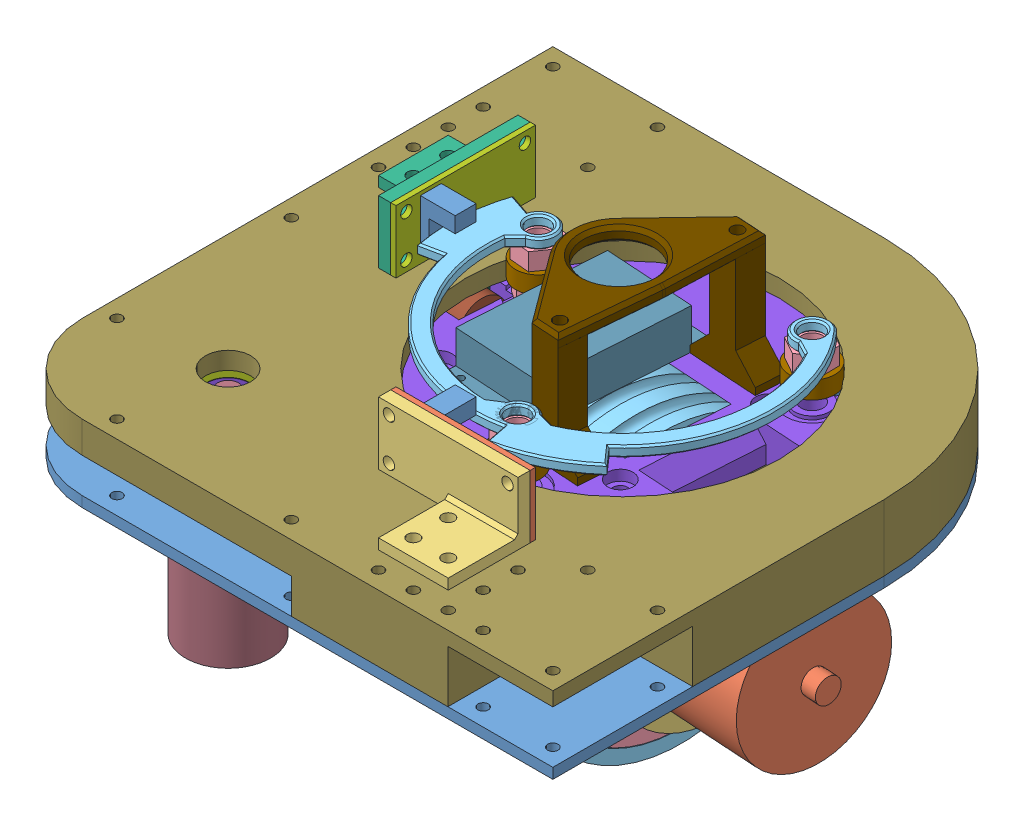
SolidWorks assembly st, configuration ﾃﾞﾌｫﾙﾄ. Lengths in mm.
Overall size (160 121.43 160).
34 component instances, 25 part files, 91 mates.
Components (placement in the parent):
- Copy of st2_base_l^st-1: Copy of st2_base_l^st [ﾃﾞﾌｫﾙﾄ] at (-18.8762 42.7582 -10) x (1 0 0) z (0 1 0) size (160 160 3) (virtual)
- Copy of Copy of 足回りモータ^st-1: Copy of Copy of 足回りモータ^st [ﾃﾞﾌｫﾙﾄ] at (-26.8603 18.2582 -10.5046) x (0 1 0) z (0.063076 0 -0.998009) size (42 98.4 42) (virtual)
- Part5^st-1: Part5^st [ﾃﾞﾌｫﾙﾄ] at (-26.8603 18.2582 -10.5046) x (0 -1 0) z (-0.998009 0 -0.063076) size (57 54 38) (virtual)
- Copy of Part1^st-1: Copy of Part1^st [ﾃﾞﾌｫﾙﾄ] at (-1.01 -10.8145 -54.8758) x (0.057768 -0.401507 -0.914032) z (-0.998009 0 -0.063076) size (72 72 12) (virtual)
- Part7^st-1: Part7^st [ﾃﾞﾌｫﾙﾄ] at (-26.6079 18.2582 -14.4966) x (0 1 0) z (0.063076 0 -0.998009) size (80 42 80) (virtual)
- Part8^st-1: Part8^st [ﾃﾞﾌｫﾙﾄ] at (-54.8045 18.2582 -12.2707) x (0.046572 -0.674423 -0.736875) z (-0.998009 0 -0.063076) size (26 26 8) (virtual)
- Part9^st-1: Part9^st [ﾃﾞﾌｫﾙﾄ] at (-54.8045 18.2582 -12.2707) x (0 -1 0) z (-0.998009 0 -0.063076) size (48 50 11) (virtual)
- Part10^st-1: Part10^st [ﾃﾞﾌｫﾙﾄ] at (-26.8603 48.2582 -10.5046) x (-0.998009 0 -0.063076) z (0 1 0) size (98.93 99.5 10) (virtual)
- Copy of Assem4^st-1: Copy of Assem4^st [ﾃﾞﾌｫﾙﾄ] at (210.0035 137.7188 42.496) x (0.981351 0 0.192225) z (-0.192225 0 0.981351) (virtual)
- Copy of Copy of Copy of Copy (3) of Part3^st-1: Copy of Copy of Copy of Copy (3) of Part3^st [ﾃﾞﾌｫﾙﾄ] at (0.121 53.2582 28.2971) x (0.124113 0.990356 -0.061566) z (0.444379 0 0.895839) size (13 13 5) (virtual)
- Copy (2) of Copy of Copy of Copy (3) of Part3^st-2: Copy (2) of Copy of Copy of Copy (3) of Part3^st [ﾃﾞﾌｫﾙﾄ] at (4.7915 53.2582 -45.6006) x (0.32156 0.922442 0.213776) z (0.55363 0 -0.832763) size (13 13 5) (virtual)
- Copy (3) of Copy of Copy of Copy (3) of Part3^st-3: Copy (3) of Copy of Copy of Copy (3) of Part3^st [ﾃﾞﾌｫﾙﾄ] at (-66.5311 53.2582 -13.0119) x (-0.024356 0.922442 0.385367) z (0.998009 0 0.063076) size (13 13 5) (virtual)
- Copy of st2_base_u^st-1: Copy of st2_base_u^st [ﾃﾞﾌｫﾙﾄ] at (-18.8762 59.7582 -10) x (1 0 0) z (0 1 0) size (160 160 19) (virtual)
- Copy of Copy of Copy of Copy (3) of Part3^st-2: Copy of Copy of Copy of Copy (3) of Part3^st [ﾃﾞﾌｫﾙﾄ] at (-55.3618 63.2582 -22.2904) x (-0.478032 0 0.878342) z (0 1 0) size (13 13 5) (virtual)
- Copy of Copy of Copy of Copy (3) of Part3^st-3: Copy of Copy of Copy of Copy (3) of Part3^st [ﾃﾞﾌｫﾙﾄ] at (10.0104 63.2582 -35.4522) x (0.874344 0 0.485306) z (0 1 0) size (13 13 5) (virtual)
- Copy of Copy of Copy of Copy (3) of Part3^st-4: Copy of Copy of Copy of Copy (3) of Part3^st [ﾃﾞﾌｫﾙﾄ] at (-11.2772 63.2582 27.7426) x (0.840503 0 0.541806) z (0 1 0) size (13 13 5) (virtual)
- Part30^st-1: Part30^st [ﾃﾞﾌｫﾙﾄ] at (-106.4764 42.7582 -41.574) x (-0.707107 0 0.707107) z (0 -1 0) size (24.4 24.4 60.8) (virtual)
- Part31^st-1: Part31^st [ﾃﾞﾌｫﾙﾄ] at (30.1273 58.2582 33.0552) x (-0.998009 0 -0.063076) z (0 1 0) size (25.8 49.4 11.5) (virtual)
- Copy of st2_stgr^st-1: Copy of st2_stgr^st [ﾃﾞﾌｫﾙﾄ] at (-37.084 1 -21.1707) x (-0.998009 0 -0.063076) z (0.063076 0 -0.998009) size (121.99 10 121.99) (virtual)
- Copy of st2_stgr2^st-1: Copy of st2_stgr2^st [ﾃﾞﾌｫﾙﾄ] at (-144.7938 -39.0873 81.6755) x (-1 0 0) z (0 0 -1) size (42 10 42) (virtual)
- Copy of Part10^st-1: Copy of Part10^st [ﾃﾞﾌｫﾙﾄ] at (-73.8405 58.2582 86.1807) x (1 0 0) z (0 -1 0) size (12 12 5) (virtual)
- Part32^st-1: Part32^st [ﾃﾞﾌｫﾙﾄ] at (-28.1078 58.2582 -10.5835) x (-0.998009 0 -0.063076) z (0 1 0) size (33.25 56 34) (virtual)
- Part33^st-1: Part33^st [ﾃﾞﾌｫﾙﾄ] at (-11.7253 224.5363 45) x (-1 0 0) z (0 0 -1) size (6 14 10) (virtual)
- Part34^st-1: Part34^st [ﾃﾞﾌｫﾙﾄ] at (12.8544 236.4656 45) size (40 18 1.5) (virtual)
- Part35^st-1: Part35^st [ﾃﾞﾌｫﾙﾄ] at (12.8544 236.4656 46.5) size (40 18 23.5) (virtual)
- Part36^st-1: Part36^st [ﾃﾞﾌｫﾙﾄ] at (10.0104 68.2582 -35.4522) x (0.874344 0 0.485306) z (0 1 0) size (11.55 10 5) (virtual)
- Part36^st-2: Part36^st [ﾃﾞﾌｫﾙﾄ] at (-11.2772 68.2582 27.7426) x (-0.959358 0 -0.282192) z (0 1 0) size (11.55 10 5) (virtual)
- Part36^st-3: Part36^st [ﾃﾞﾌｫﾙﾄ] at (-55.3618 68.2582 -22.2904) x (-0.995821 0 -0.091329) z (0 1 0) size (11.55 10 5) (virtual)
- Part37^st-1: Part37^st [ﾃﾞﾌｫﾙﾄ] at (10.0104 73.2582 -35.4522) x (0.933273 0 -0.359167) z (0 1 0) size (54.96 68.38 3) (virtual)
- Copy of Part35^st-1: Copy of Part35^st [ﾃﾞﾌｫﾙﾄ] at (-75.3762 236.4656 1.7306) x (0 0 1) z (-1 0 0) size (40 18 23.5) (virtual)
- Part33^st-2: Part33^st [ﾃﾞﾌｫﾙﾄ] at (-73.8762 224.5363 -2.8492) x (0 0 -1) z (1 0 0) size (6 14 10) (virtual)
- Copy of Part34^st-1: Copy of Part34^st [ﾃﾞﾌｫﾙﾄ] at (-73.8762 236.4656 1.7306) x (0 0 1) z (-1 0 0) size (40 18 1.5) (virtual)
- Part37^st-3: Part37^st [ﾃﾞﾌｫﾙﾄ] at (-11.2772 73.2582 27.7426) x (-0.155589 0 0.987822) z (0 1 0) size (54.96 68.38 3) (virtual)
- Part36^st-4: Part36^st [ﾃﾞﾌｫﾙﾄ] at (-55.3618 58.2582 -22.2904) x (-0.908527 0 0.417826) z (0 1 0) size (11.55 10 5) (virtual)
Mates (geometry in assembly coordinates):
- 相対固定5: in place: plane of ? through (-112.9944 -0.3949 73.4466) normal (0.707107 0 0.707107); plane of ? through (-19.7739 0 -19.7739) normal (0.707107 0 0.707107); moOrthogonalPlaneRef_w of ? through (-112.9944 -0.3949 73.4466) normal (0.707107 0 0.707107); plane of ? through (-19.7739 0 -19.7739) normal (0 1 0); plane of ? through (-112.9944 -0.3949 73.4466) normal (0.707107 0 0.707107); plane of ? through (-19.7739 0 -19.7739) normal (0.707107 0 -0.707107); plane of Copy of Copy of 足回りモータ^st-1 through (-26.8603 18.2582 -10.5046) normal (-0.998009 0 -0.063076); unknown of Part5^st-1
- 一致27: coincident aligned: plane of ?; plane of ?
- 一致28: coincident aligned: moOrthogonalPlaneRef_w of Copy of Copy of 足回りモータ^st2-1; plane of Part5^st2-1 through (-26.8603 18.2582 -10.5046) normal (-0.063076 0 0.998009)
- 一致29: coincident anti-aligned: moOrthogonalPlaneRef_w of Copy of Copy of 足回りモータ^st2-1; plane of Part5^st2-1 through (-26.8603 18.2582 -10.5046) normal (0 -1 0)
- 同心円16: concentric anti-aligned: cylinder of Part5^st2-1 through (8.0701 18.2582 -8.2969) axis (-0.998009 0 -0.063076) radius 25; cylinder of Copy of Part1^st2-1 through (-15.8822 18.2582 -9.8108) axis (0.998009 0 0.063076) radius 25
- 相対固定7: in place: plane of ? through (-22.8566 -14.0328 -4.7881) normal (0 -1 0); plane of ? through (0 -14.0328 0) normal (0 -1 0); plane of ? through (-22.8566 -14.0328 -4.7881) normal (0 -1 0); plane of ? through (0 -14.0328 0) normal (0 0 -1); plane of ? through (-22.8566 -14.0328 -4.7881) normal (0 -1 0); plane of ? through (0 -14.0328 0) normal (-1 0 0); plane of Copy of Copy of 足回りモータ^st-1 through (-26.6079 18.2582 -14.4966) normal (0.063076 0 -0.998009); unknown of Part7^st-1
- 一致34: coincident aligned: plane of ?; plane of ?
- 一致35: coincident aligned: moOrthogonalPlaneRef_w of Copy of Copy of 足回りモータ^st2-1; plane of Part7^st2-1 through (-26.6079 18.2582 -14.4966) normal (0.998009 0 0.063076)
- 一致36: coincident anti-aligned: moOrthogonalPlaneRef_w of Copy of Copy of 足回りモータ^st2-1; plane of Part7^st2-1 through (-26.6079 18.2582 -14.4966) normal (0 1 0)
- 一致37: coincident anti-aligned: plane of Copy of Part1^st2-1 through (-15.8822 18.2582 -9.8108) normal (-0.998009 0 -0.063076); plane of Part7^st2-1 through (-15.6299 18.2582 -13.8028) normal (0.998009 0 0.063076)
- 同心円19: concentric anti-aligned: cylinder of Copy of Copy of 足回りモータ^st2-1 through (-54.1059 18.2582 -12.2266) axis (0.998009 0 0.063076) radius 5; cylinder of Part8^st2-1 through (-46.8204 18.2582 -11.7661) axis (-0.998009 0 -0.063076) radius 5
- 距離1: distance = 45 mm anti-aligned: plane of Part5^st2-1 through (-1.91 18.2582 -8.9277) normal (-0.998009 0 -0.063076); plane of Part9^st2-1 through (-46.8204 18.2582 -11.7661) normal (0.998009 0 0.063076)
- 相対固定10: in place: plane of ? through (-74.4978 -5.5664 18.4032) normal (-0.707107 0 0.707107); plane of ? through (-46.4505 0 46.4505) normal (-0.707107 0 0.707107); plane of ? through (-74.4978 -5.5664 18.4032) normal (-0.707107 0 0.707107); plane of ? through (-46.4505 0 46.4505) normal (0 1 0); plane of ? through (-74.4978 -5.5664 18.4032) normal (-0.707107 0 0.707107); plane of ? through (-46.4505 0 46.4505) normal (0.707107 0 0.707107); plane of Part5^st-1 through (-1.91 48.2582 -8.9277) normal (0 1 0); unknown of Part10^st-1
- 一致44: coincident aligned: plane of ?; plane of ?
- 一致45: coincident aligned: moOrthogonalPlaneRef_w of Part5^st2-1; plane of Part10^st2-1 through (-26.8603 48.2582 -10.5046) normal (-0.063076 0 0.998009)
- 一致46: coincident anti-aligned: moOrthogonalPlaneRef_w of Part5^st2-1; plane of Part10^st2-1 through (-26.8603 48.2582 -10.5046) normal (-0.998009 0 -0.063076)
- 同心円20: concentric aligned: cylinder of Copy of st2_base_l^st2-1 through (-18.8762 45.7582 -10) axis (0 -1 0) radius 45; cylinder of Part10^st2-1 through (-18.8762 58.2582 -10) axis (0 -1 0) radius 49.75
- 同心円21: concentric aligned: cylinder of Part8^st2-1 through (-46.8204 18.2582 -11.7661) axis (-0.998009 0 -0.063076) radius 13; cylinder of Part9^st2-1 through (-46.8204 18.2582 -11.7661) axis (-0.998009 0 -0.063076) radius 13.15
- 一致52: coincident anti-aligned: plane of Part8^st2-1 through (-54.8045 18.2582 -12.2707) normal (-0.998009 0 -0.063076); plane of Part9^st2-1 through (-54.8045 18.2582 -12.2707) normal (0.998009 0 0.063076)
- 平行1: parallel aligned: plane of Part5^st2-1 through (-0.207 18.2582 -35.8739) normal (0.063076 0 -0.998009); plane of Part9^st2-1 through (-56.6632 48.2582 -30.4241) normal (0.063076 0 -0.998009)
- 同心円22: concentric aligned: circle of Part10^st2-1; unknown of Copy of Assem4^st2-1/steeri_gear-1
- 同心円24: concentric aligned: cylinder of Part10^st2-1 through (2.3429 53.2582 32.7763) axis (-0.444379 0 -0.895839) radius 2.9; cylinder of Copy of Copy of Copy of Copy (3) of Part3^st2-1 through (2.3429 53.2582 32.7763) axis (-0.444379 0 -0.895839) radius 3
- 一致57: coincident aligned: plane of Part10^st2-1 through (2.3429 53.2582 32.7763) normal (0.444379 0 0.895839); plane of Copy of Copy of Copy of Copy (3) of Part3^st2-1 through (2.3429 53.2582 32.7763) normal (0.444379 0 0.895839)
- 同心円25: concentric aligned: cylinder of Part10^st2-1 through (7.5596 53.2582 -49.7644) axis (-0.55363 0 0.832763) radius 2.9; cylinder of Copy (2) of Copy of Copy of Copy (3) of Part3^st2-2 through (7.5596 53.2582 -49.7644) axis (-0.55363 0 0.832763) radius 3
- 一致58: coincident aligned: plane of Part10^st2-1 through (7.5596 53.2582 -49.7644) normal (0.55363 0 -0.832763); plane of Copy (2) of Copy of Copy of Copy (3) of Part3^st2-2 through (7.5596 53.2582 -49.7644) normal (0.55363 0 -0.832763)
- 同心円26: concentric anti-aligned: cylinder of Part10^st2-1 through (-66.5311 53.2582 -13.0119) axis (0.998009 0 0.063076) radius 2.9; cylinder of Copy (3) of Copy of Copy of Copy (3) of Part3^st2-3 through (-61.5411 53.2582 -12.6965) axis (-0.998009 0 -0.063076) radius 3
- 一致59: coincident aligned: plane of Part10^st2-1 through (-66.5311 53.2582 -13.0119) normal (-0.998009 0 -0.063076); plane of Copy (3) of Copy of Copy of Copy (3) of Part3^st2-3 through (-66.5311 53.2582 -13.0119) normal (-0.998009 0 -0.063076)
- 同心円27: concentric aligned: cylinder of Part10^st2-1 through (-18.8762 58.2582 -10) axis (0 -1 0) radius 49.75; cylinder of Copy of Copy of Part9^st2-1 through (-18.8762 64.7582 -10) axis (0 -1 0) radius 45
- 正接2: tangent anti-aligned: cylinder of Copy (2) of Copy of Copy of Copy (3) of Part3^st2-2 through (7.5596 53.2582 -49.7644) axis (-0.55363 0 0.832763) radius 6.5; plane of Copy of Copy of Part9^st2-1 through (-18.8762 59.7582 -10) normal (0 -1 0)
- 平行3: parallel aligned: plane of Copy of st2_base_l^st2-1 through (51.1238 45.7582 -80) normal (0 0 -1); plane of Copy of Copy of Part9^st2-1 through (51.1238 64.7582 -80) normal (0 0 -1)
- 同心円28: concentric anti-aligned: cylinder of Copy of Copy of Copy of Copy (3) of Part3^st2-2 through (-55.3618 68.2582 -22.2904) axis (0 -1 0) radius 3; cylinder of Part10^st2-1 through (-55.3618 48.2572 -22.2904) axis (0 1 0) radius 3.15
- 同心円29: concentric anti-aligned: cylinder of Copy of Copy of Copy of Copy (3) of Part3^st2-3 through (10.0104 68.2582 -35.4522) axis (0 -1 0) radius 3; cylinder of Part10^st2-1 through (10.0104 48.2572 -35.4522) axis (0 1 0) radius 3.15
- 同心円30: concentric anti-aligned: cylinder of Copy of Copy of Copy of Copy (3) of Part3^st2-4 through (-11.2772 68.2582 27.7426) axis (0 -1 0) radius 3; cylinder of Part10^st2-1 through (-11.2772 48.2572 27.7426) axis (0 1 0) radius 3.15
- 同心円38: concentric aligned: cylinder of Copy of st2_base_l^st2-1 through (-75.4447 45.7582 46.5685) axis (0 -1 0) radius 6.5; cylinder of Part30^st2-1 through (-75.4447 44.7582 46.5685) axis (0 -1 0) radius 6.5
- 同心円39: concentric anti-aligned: cylinder of Copy of st2_base_l^st2-1 through (-82.1622 45.7582 39.851) axis (0 -1 0) radius 1.5; cylinder of Part30^st2-1 through (-82.1622 37.7582 39.851) axis (0 1 0) radius 1.5
- 一致77: coincident anti-aligned: plane of Copy of st2_base_l^st2-1 through (-18.8762 42.7582 -10) normal (0 -1 0); plane of Part30^st2-1 through (-75.4447 42.7582 46.5685) normal (0 1 0)
- 一致81: coincident anti-aligned: plane of Part10^st2-1 through (-18.8762 58.2582 -10) normal (0 1 0); plane of Part31^st2-1 through (30.1273 58.2582 33.0552) normal (0 -1 0)
- 同心円43: concentric aligned: cylinder of Copy of st2_stgr2^st2-1 through (-75.4447 53.2582 46.5685) axis (0 1 0) radius 6.15; cylinder of Copy of Part10^st2-1 through (-75.4447 53.2582 46.5685) axis (0 1 0) radius 6
- 同心円47: concentric anti-aligned: cylinder of Copy of st2_stgr2^st2-1 through (-54.4461 55.7582 46.5685) axis (-1 0 0) radius 1.65; cylinder of Copy of Part10^st2-1 through (-81.4457 55.7582 46.5685) axis (1 0 0) radius 1.5
- 同心円48: concentric anti-aligned: cylinder of Part30^st2-1 through (-75.4447 59.7582 46.5685) axis (0 -1 0) radius 3; cylinder of Copy of Part10^st2-1 through (-75.4447 53.2582 46.5685) axis (0 1 0) radius 3
- 一致84: coincident aligned: plane of Part10^st2-1 through (-18.8762 58.2582 -10) normal (0 1 0); plane of st2_stgr2-1 through (-75.4447 58.2582 46.5685) normal (0 1 0)
- 同心円49: concentric aligned: cylinder of Part10^st2-1 through (-18.8762 58.2582 -10) axis (0 -1 0) radius 49.75; cylinder of st2_stgr-1 through (-18.8762 98.2583 -10) axis (0 -1 0) radius 50
- 平行6: parallel anti-aligned: plane of Part10^st2-1 through (-12.7631 48.2582 -1.1327) normal (-0.832763 0 -0.55363); plane of st2_stgr-1 through (-11.0625 48.2582 -3.8713) normal (0.832763 0 0.55363)
- 距離2: distance = 14 mm anti-aligned: plane of Copy of st2_base_l^st2-1 through (-18.8762 45.7582 -10) normal (0 1 0); plane of Copy of Copy of Part9^st2-1 through (-18.8762 59.7582 -10) normal (0 -1 0)
- 同心円50: concentric aligned: cylinder of Part10^st2-1 through (-9.3783 48.2582 -33.4476) axis (0 1 0) radius 1.75; cylinder of Part32^st2-1 through (-9.3783 58.2582 -33.4476) axis (0 1 0) radius 1.75
- 平行7: parallel aligned: plane of Part10^st2-1 through (7.1239 48.2572 6.6732) normal (0.998009 0 0.063076); plane of Part32^st2-1 through (-5.6386 88.2582 -29.2033) normal (0.998009 0 0.063076)
- 一致89: coincident anti-aligned: plane of Part10^st2-1 through (-18.8762 58.2582 -10) normal (0 1 0); plane of Part32^st2-1 through (-28.1078 58.2582 -10.5835) normal (0 -1 0)
- 相対固定15: in place: plane of ? through (-6.9896 101.9468 -42.8084) normal (0 -1 0); plane of ? through (0 101.9468 0) normal (0 -1 0); plane of ? through (-6.9896 101.9468 -42.8084) normal (0 -1 0); plane of ? through (0 101.9468 0) normal (0 0 -1); plane of ? through (-6.9896 101.9468 -42.8084) normal (0 -1 0); plane of ? through (0 101.9468 0) normal (-1 0 0); plane of Part34^st-1 through (12.8544 236.4656 46.5) normal (0 0 1); unknown of Part35^st-1
- 一致96: coincident aligned: plane of ?; plane of ?
- 一致97: coincident aligned: moOrthogonalPlaneRef_w of Part34^st2-1; plane of Part35^st2-1 through (12.8544 236.4656 46.5) normal (0 1 0)
- 一致98: coincident anti-aligned: unknown of Part34^st2-1; plane of Part35^st2-1 through (12.8544 236.4656 46.5) normal (1 0 0)
- 平行9: parallel anti-aligned: plane of Copy of st2_base_u^st2-1 through (51.1238 64.7582 80) normal (0 0 1); plane of Part34^st2-1 through (12.8544 236.4656 45) normal (0 0 -1)
- 一致99: coincident anti-aligned: plane of Part33^st2-1 through (-11.7253 224.5363 45) normal (0 0 1); plane of Part34^st2-1 through (12.8544 236.4656 45) normal (0 0 -1)
- 平行10: parallel anti-aligned: plane of Copy of st2_base_u^st2-1 through (-18.8762 64.7582 -10) normal (0 1 0); plane of Part33^st2-1 through (-15.8762 67.7582 35) normal (0 -1 0)
- 距離5: distance = 7 mm aligned: plane of Part33^st2-1 through (-21.8762 81.7582 35) normal (-1 0 0); plane of Part34^st2-1 through (-28.8762 82.7582 46.5) normal (-1 0 0)
- 正接3: tangent anti-aligned: cylinder of Copy of st2_base_u^st2-1 through (-18.8762 64.7582 -10) axis (0 -1 0) radius 45; plane of Part33^st2-1 through (-11.7253 224.5363 35) normal (0 0 -1)
- 距離6: distance = 1 mm aligned: plane of Part34^st2-1 through (11.1238 82.7582 46.5) normal (0 1 0); plane of Part33^st2-1 through (-15.8762 81.7582 35) normal (0 1 0)
- 一致101: coincident anti-aligned: plane of Copy of st2_base_u^st2-1 through (-18.8762 64.7582 -10) normal (0 1 0); plane of Part35^st2-1 through (-28.8762 64.7582 50) normal (0 -1 0)
- 同心円52: concentric aligned: cylinder of Copy of st2_base_u^st2-1 through (6.1238 59.7572 65) axis (0 1 0) radius 1.5; cylinder of Part35^st2-1 through (6.1238 64.7572 65) axis (0 1 0) radius 1.75
- 相対固定16: in place: plane of ? through (8.3474 64.2582 17.2236) normal (0 1 0); plane of ? through (0 64.2582 0) normal (0 1 0); plane of ? through (8.3474 64.2582 17.2236) normal (0 1 0); plane of ? through (0 64.2582 0) normal (0 0 -1); plane of ? through (8.3474 64.2582 17.2236) normal (0 1 0); plane of ? through (0 64.2582 0) normal (1 0 0); plane of Copy of Copy of Copy of Copy (3) of Part3^st-3 through (10.0104 68.2582 -35.4522) normal (0 1 0); unknown of Part36^st-1
- 一致106: coincident aligned: plane of ?; plane of ?
- 一致107: coincident aligned: moOrthogonalPlaneRef_w of Copy of Copy of Copy of Copy (3) of Part3^st2-3; plane of Part36^st2-1 through (10.0104 68.2582 -35.4522) normal (0.485306 0 -0.874344)
- 一致108: coincident anti-aligned: moOrthogonalPlaneRef_w of Copy of Copy of Copy of Copy (3) of Part3^st2-3; plane of Part36^st2-1 through (10.0104 68.2582 -35.4522) normal (0.874344 0 0.485306)
- 同心円53: concentric aligned: cylinder of Copy of Copy of Copy of Copy (3) of Part3^st2-4 through (-11.2772 68.2582 27.7426) axis (0 -1 0) radius 3; cylinder of Part36^st2-2 through (-11.2772 73.2582 27.7426) axis (0 -1 0) radius 3
- 一致109: coincident anti-aligned: plane of Copy of Copy of Copy of Copy (3) of Part3^st2-4 through (-11.2772 68.2582 27.7426) normal (0 1 0); plane of Part36^st2-2 through (-11.2772 68.2582 27.7426) normal (0 -1 0)
- 同心円54: concentric aligned: cylinder of Copy of Copy of Copy of Copy (3) of Part3^st2-2 through (-55.3618 68.2582 -22.2904) axis (0 -1 0) radius 3; cylinder of Part36^st2-3 through (-55.3618 73.2582 -22.2904) axis (0 -1 0) radius 3
- 一致110: coincident anti-aligned: plane of Copy of Copy of Copy of Copy (3) of Part3^st2-2 through (-55.3618 68.2582 -22.2904) normal (0 1 0); plane of Part36^st2-3 through (-55.3618 68.2582 -22.2904) normal (0 -1 0)
- 同心円56: concentric aligned: cylinder of Part36^st2-1 through (10.0104 73.2582 -35.4522) axis (0 -1 0) radius 3; cylinder of Part37^st2-1 through (10.0104 74.2582 -35.4522) axis (0 -1 0) radius 3.15
- 同心円57: concentric anti-aligned: cylinder of Part36^st2-2 through (-11.2772 73.2582 27.7426) axis (0 -1 0) radius 3; cylinder of Part37^st2-1 through (-11.2772 73.2582 27.7426) axis (0 1 0) radius 3.15
- 一致114: coincident anti-aligned: plane of Part36^st2-1 through (10.0104 73.2582 -35.4522) normal (0 1 0); plane of Part37^st2-1 through (10.0104 73.2582 -35.4522) normal (0 -1 0)
- 距離7: distance = 1 mm aligned: plane of Copy of Part34^st2-1 through (-75.3762 82.7582 0) normal (0 1 0); plane of Part33^st2-2 through (-63.8762 81.7582 -7) normal (0 1 0)
- 距離8: distance = 7 mm aligned: plane of Part33^st2-2 through (-63.8762 81.7582 -7) normal (0 0 1); plane of Copy of Part34^st2-1 through (-75.3762 82.7582 0) normal (0 0 1)
- 一致115: coincident anti-aligned: plane of Part33^st2-2 through (-73.8762 224.5363 -2.8492) normal (-1 0 0); plane of Copy of Part34^st2-1 through (-73.8762 236.4656 1.7306) normal (1 0 0)
- 相対固定17: in place: plane of ? through (-42.5975 304.1492 -77.7427) normal (0 0 1); plane of ? through (-42.5975 304.1492 -77.7427) normal (0 0 1); plane of ? through (-42.5975 304.1492 -77.7427) normal (0 1 0); line of ? through (-42.5975 304.1492 -77.7427) axis (0 1 0); plane of ? through (-42.5975 304.1492 -77.7427) normal (1 0 0); line of ? through (-42.5975 304.1492 -77.7427) axis (-1 0 0); plane of Copy of Part35^st-1 through (-75.3762 236.4656 1.7306) normal (-1 0 0); unknown of Copy of Part34^st-1
- 一致116: coincident aligned: plane of ?; plane of ?
- 一致117: coincident aligned: plane of Copy of Part35^st2-1 through (-75.3762 236.4656 1.7306) normal (0 1 0); moOrthogonalPlaneRef_w of Copy of Part34^st2-1 through (-75.3762 236.4656 1.7306) normal (0 1 0)
- 一致118: coincident anti-aligned: plane of Copy of Part35^st2-1 through (-75.3762 236.4656 1.7306) normal (0 0 1); moOrthogonalPlaneRef_w of Copy of Part34^st2-1 through (236.4656 1.7306 0) axis (0 -1 0)
- 同心円58: concentric aligned: cylinder of Copy of st2_base_u^st2-1 through (-83.8762 59.7572 -25) axis (0 1 0) radius 1.5; cylinder of Copy of Part35^st2-1 through (-83.8762 64.7572 -25) axis (0 1 0) radius 1.75
- 同心円59: concentric aligned: cylinder of Copy of st2_base_u^st2-1 through (-93.8762 59.7572 -25) axis (0 1 0) radius 1.5; cylinder of Copy of Part35^st2-1 through (-93.8762 64.7572 -25) axis (0 1 0) radius 1.75
- 一致119: coincident anti-aligned: plane of Copy of st2_base_u^st2-1 through (-18.8762 64.7582 -10) normal (0 1 0); plane of Copy of Part35^st2-1 through (-78.8762 64.7582 -40) normal (0 -1 0)
- 同心円62: concentric aligned: cylinder of Part36^st2-2 through (-11.2772 73.2582 27.7426) axis (0 -1 0) radius 3; cylinder of Part37^st2-3 through (-11.2772 74.2582 27.7426) axis (0 -1 0) radius 3.15
- 同心円63: concentric anti-aligned: cylinder of Part36^st2-3 through (-55.3618 73.2582 -22.2904) axis (0 -1 0) radius 3; cylinder of Part37^st2-3 through (-55.3618 73.2582 -22.2904) axis (0 1 0) radius 3.15
- 一致121: coincident anti-aligned: plane of Part36^st2-3 through (-55.3618 73.2582 -22.2904) normal (0 1 0); plane of Part37^st2-3 through (-11.2772 73.2582 27.7426) normal (0 -1 0)
- 一致122: coincident anti-aligned: plane of Part10^st2-1 through (-26.8603 56.2582 -10.5046) normal (0 -1 0); plane of st2_stgr-1 through (-37.084 56.2582 -21.1707) normal (0 1 0)
- 同心円64: concentric aligned: cylinder of Part10^st2-1 through (-23.4387 48.2572 -32.9335) axis (0 1 0) radius 1.15; cylinder of Part31^st2-1 through (-23.4387 58.2572 -32.9335) axis (0 1 0) radius 1
- 同心円65: concentric aligned: cylinder of Part10^st2-1 through (-41.4029 48.2572 -34.0688) axis (0 1 0) radius 1.15; cylinder of Part31^st2-1 through (-41.4029 58.2572 -34.0688) axis (0 1 0) radius 1
- 同心円66: concentric anti-aligned: cylinder of Part10^st2-1 through (-55.3618 48.2572 -22.2904) axis (0 1 0) radius 3.15; cylinder of Part36^st2-4 through (-55.3618 63.2582 -22.2904) axis (0 -1 0) radius 3
- 一致123: coincident anti-aligned: plane of Copy of Copy of Copy of Copy (3) of Part3^st2-2 through (-55.3618 63.2582 -22.2904) normal (0 -1 0); plane of Part36^st2-4 through (-55.3618 63.2582 -22.2904) normal (0 1 0)
- 一致124: coincident anti-aligned: plane of Part10^st2-1 through (-55.3618 58.2582 -22.2904) normal (0 1 0); plane of Part36^st2-4 through (-55.3618 58.2582 -22.2904) normal (0 -1 0)
- 一致125: coincident aligned: plane of Part37^st2-1 through (10.0104 76.2582 -35.4522) normal (0 1 0); plane of Part37^st2-3 through (-11.2772 76.2582 27.7426) normal (0 1 0)
- 一致126: coincident anti-aligned: plane of Part36^st2-2 through (-11.2772 73.2582 27.7426) normal (0 1 0); plane of Part37^st2-1 through (10.0104 73.2582 -35.4522) normal (0 -1 0)
